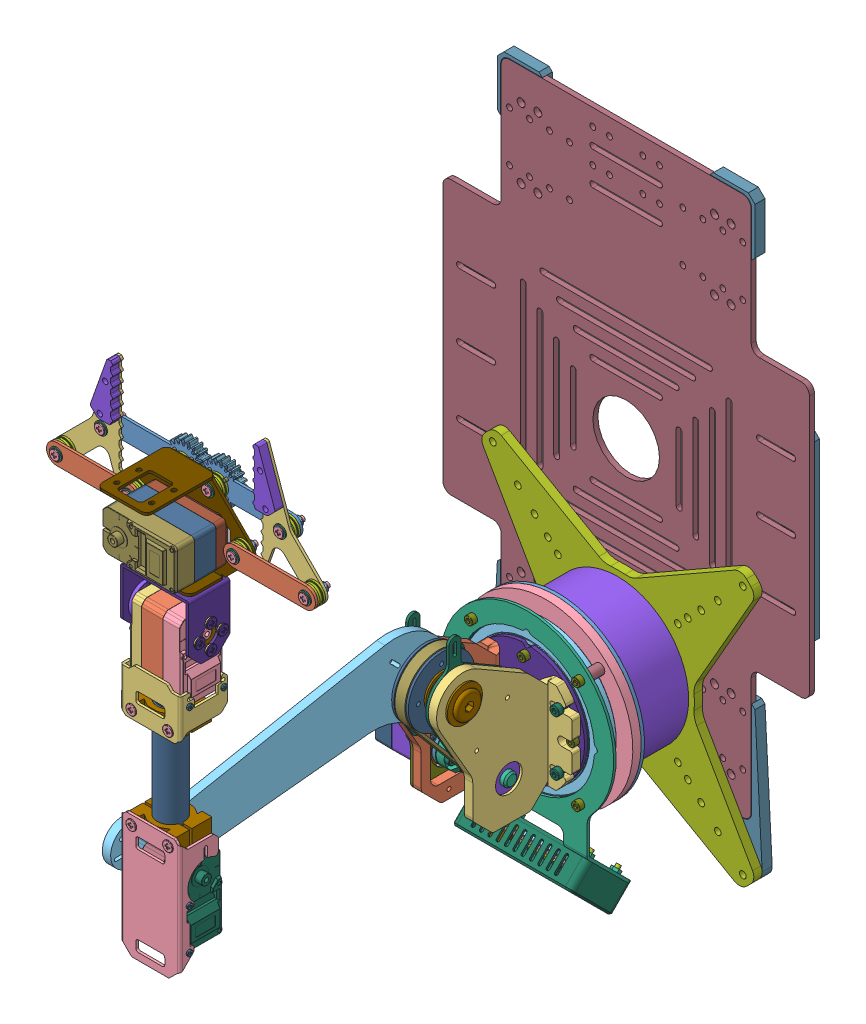
SolidWorks assembly RoArm-M1 STEP, configuration Default. Lengths in mm. (continued)
Components (placement in the parent): (continued)
- RoArm-M1 STEP(2)^RoArm-M1 STEP-1: RoArm-M1 STEP(2)^RoArm-M1 STEP [Default] at origin size (176.32 372.07 316.7) (virtual) (continued)
  - 银色金属螺丝 M2x8^RoArm-M1 STEP(2)_RoArm-M1 STEP-4: 银色金属螺丝 M2x8^RoArm-M1 STEP(2)_RoArm-M1 STEP [Default] at (19.3974 240.0016 262.6404) x (1 0 0) z (0 0 -1) size (3.6 3.6 9.22) (virtual)
  - 银色金属螺丝 M2x8^RoArm-M1 STEP(2)_RoArm-M1 STEP-5: 银色金属螺丝 M2x8^RoArm-M1 STEP(2)_RoArm-M1 STEP [Default] at (8.5797 240.0016 262.6404) x (1 0 0) z (0 0 -1) size (3.6 3.6 9.22) (virtual)
  - 银色金属螺丝 M2x8^RoArm-M1 STEP(2)_RoArm-M1 STEP-6: 银色金属螺丝 M2x8^RoArm-M1 STEP(2)_RoArm-M1 STEP [Default] at (-1.6026 229.8193 262.6404) x (1 0 0) z (0 0 -1) size (3.6 3.6 9.22) (virtual)
  - 银色金属螺丝 M2x8^RoArm-M1 STEP(2)_RoArm-M1 STEP-7: 银色金属螺丝 M2x8^RoArm-M1 STEP(2)_RoArm-M1 STEP [Default] at (8.5797 229.8193 262.6404) x (1 0 0) z (0 0 -1) size (3.6 3.6 9.22) (virtual)
  - 银色金属螺丝 M2x8^RoArm-M1 STEP(2)_RoArm-M1 STEP-8: 银色金属螺丝 M2x8^RoArm-M1 STEP(2)_RoArm-M1 STEP [Default] at (-1.6026 240.0016 262.6404) x (1 0 0) z (0 0 -1) size (3.6 3.6 9.22) (virtual)
  - 弹性垫片 M3^RoArm-M1 STEP(2)_RoArm-M1 STEP-24: 弹性垫片 M3^RoArm-M1 STEP(2)_RoArm-M1 STEP [Default] at (7 0 48.12) size (5.2 5.2 0.88) (virtual)
  - 弹性垫片 M3^RoArm-M1 STEP(2)_RoArm-M1 STEP-25: 弹性垫片 M3^RoArm-M1 STEP(2)_RoArm-M1 STEP [Default] at (0 -7 48.12) size (5.2 5.2 0.88) (virtual)
  - 弹性垫片 M3^RoArm-M1 STEP(2)_RoArm-M1 STEP-26: 弹性垫片 M3^RoArm-M1 STEP(2)_RoArm-M1 STEP [Default] at (-7 0 48.12) size (5.2 5.2 0.88) (virtual)
  - 弹性垫片 M3^RoArm-M1 STEP(2)_RoArm-M1 STEP-27: 弹性垫片 M3^RoArm-M1 STEP(2)_RoArm-M1 STEP [Default] at (0 7 48.12) size (5.2 5.2 0.88) (virtual)
  - 弹性垫片 M3^RoArm-M1 STEP(2)_RoArm-M1 STEP-28: 弹性垫片 M3^RoArm-M1 STEP(2)_RoArm-M1 STEP [Default] at (0 0 44.32) size (5.2 5.2 0.88) (virtual)
- vertical tool-1: vertical tool [Default] at (17.9615 -304.3961 -7.6382) x (0 1 0) z (1 0 0) size (68.1 225.29 14) (hidden)
- moebius_base_2-1: moebius_base_2 [Default] at (75.4807 148.9605 -3) x (0 1 0) z (0 0 1) size (324 220 3)
- bumper_roarm-1: bumper_roarm [Default] at (75.4807 148.9605 -3) x (0 -1 0) z (0 0 -1) size (357.68 220 6)
- display protector-1: display protector [Default] at (18.4653 807.4745 926.2172) x (0 -0.707107 -0.707107) z (0 -0.707107 0.707107) size (36.8 72 17.1)
Mates (geometry in assembly coordinates):
- InPlace1: in place: plane of RoArm-M1 STEP(2)^RoArm-M1 STEP-1/大扭矩云台模块^RoArm-M1 STEP(2)_RoArm-M1 STEP-1/云台从动侧^大扭矩云台模块_RoArm-M1 STEP(2)_RoArm-M1 STEP-1 through (17.9615 10.865 89.375) normal (1 0 0); plane of ? through (17.9615 0 0) normal (1 0 0); moOrthogonalPlaneRef_w of RoArm-M1 STEP(2)^RoArm-M1 STEP-1/大扭矩云台模块^RoArm-M1 STEP(2)_RoArm-M1 STEP-1/云台从动侧^大扭矩云台模块_RoArm-M1 STEP(2)_RoArm-M1 STEP-1 through (17.9615 10.865 89.375) normal (1 0 0); plane of ? through (17.9615 0 0) normal (0 1 0); plane of RoArm-M1 STEP(2)^RoArm-M1 STEP-1/大扭矩云台模块^RoArm-M1 STEP(2)_RoArm-M1 STEP-1/云台从动侧^大扭矩云台模块_RoArm-M1 STEP(2)_RoArm-M1 STEP-1 through (17.9615 10.865 89.375) normal (1 0 0); plane of ? through (17.9615 0 0) normal (0 0 -1); plane of RoArm-M1 STEP(2)^RoArm-M1 STEP-1/大扭矩云台模块^RoArm-M1 STEP(2)_RoArm-M1 STEP-1/云台从动侧^大扭矩云台模块_RoArm-M1 STEP(2)_RoArm-M1 STEP-1 through (17.9615 10.865 89.375) normal (1 0 0); unknown of vertical tool-1
- Coincident1: coincident aligned: plane of ?; plane of ?
- Coincident2: coincident aligned: moOrthogonalPlaneRef_w of RoArm-M1 STEP(2)^RoArm-M1 STEP-1/大扭矩云台模块^RoArm-M1 STEP(2)_RoArm-M1 STEP-1/云台从动侧^大扭矩云台模块_RoArm-M1 STEP(2)_RoArm-M1 STEP-1 through (17.9615 -304.3961 -7.6382) normal (0 0 1); plane of Part135^RoArm-M1 STEP-1 through (17.9615 -304.3961 -7.6382) normal (0 0 1)
- Coincident3: coincident anti-aligned: moOrthogonalPlaneRef_w of RoArm-M1 STEP(2)^RoArm-M1 STEP-1/大扭矩云台模块^RoArm-M1 STEP(2)_RoArm-M1 STEP-1/云台从动侧^大扭矩云台模块_RoArm-M1 STEP(2)_RoArm-M1 STEP-1 through (17.9615 -304.3961 -7.6382) normal (0 -1 0); plane of Part135^RoArm-M1 STEP-1 through (17.9615 -304.3961 -7.6382) normal (0 1 0)
- Coincident1: coincident anti-aligned: plane of RoArm-M1 STEP(2)^RoArm-M1 STEP-1/X型底座^RoArm-M1 STEP(2)_RoArm-M1 STEP-1 through (0 0 0) normal (0 0 -1); plane of moebius_base_2-1 through (-70 -45.25 0) normal (0 0 1)
- Concentric1: concentric anti-aligned: cylinder of RoArm-M1 STEP(2)^RoArm-M1 STEP-1/X型底座^RoArm-M1 STEP(2)_RoArm-M1 STEP-1 through (50 50 0) axis (0 0 1) radius 2; cylinder of moebius_base_2-1 through (50 50 0) axis (0 0 -1) radius 1.75
- Concentric2: concentric anti-aligned: cylinder of RoArm-M1 STEP(2)^RoArm-M1 STEP-1/X型底座^RoArm-M1 STEP(2)_RoArm-M1 STEP-1 through (-50 50 0) axis (0 0 1) radius 2; cylinder of moebius_base_2-1 through (-50 50 0) axis (0 0 -1) radius 1.75
- InPlace2: in place: plane of moebius_base_2-1 through (-70 -45.25 -3) normal (0 0 -1); plane of ? through (0 0 -3) normal (0 0 -1); plane of moebius_base_2-1 through (-70 -45.25 -3) normal (0 0 -1); plane of ? through (0 0 -3) normal (0 1 0); plane of moebius_base_2-1 through (-70 -45.25 -3) normal (0 0 -1); plane of ? through (0 0 -3) normal (-1 0 0); plane of moebius_base_2-1 through (-70 -45.25 -3) normal (0 0 -1); unknown of bumper_roarm-1
- Coincident2: coincident aligned: plane of ?; plane of ?
- Coincident3: coincident aligned: moOrthogonalPlaneRef_w of moebius_base_2-1 through (75.4807 148.9605 -3) normal (-1 0 0); plane of bumper_roarm-1 through (75.4807 148.9605 -3) normal (-1 0 0)
- Coincident4: coincident anti-aligned: moOrthogonalPlaneRef_w of moebius_base_2-1 through (75.4807 148.9605 -3) normal (0 1 0); plane of bumper_roarm-1 through (75.4807 148.9605 -3) normal (0 -1 0)
- InPlace3: in place: plane of RoArm-M1 STEP(2)^RoArm-M1 STEP-1/中心外侧PCB支架^RoArm-M1 STEP(2)_RoArm-M1 STEP-1 through (0 -33.6427 85.1) normal (0 -0.707107 0.707107); plane of ? through (0 -59.3713 59.3713) normal (0 -0.707107 0.707107); plane of RoArm-M1 STEP(2)^RoArm-M1 STEP-1/中心外侧PCB支架^RoArm-M1 STEP(2)_RoArm-M1 STEP-1 through (0 -33.6427 85.1) normal (0 -0.707107 0.707107); plane of ? through (0 -59.3713 59.3713) normal (0 0.707107 0.707107); plane of RoArm-M1 STEP(2)^RoArm-M1 STEP-1/中心外侧PCB支架^RoArm-M1 STEP(2)_RoArm-M1 STEP-1 through (0 -33.6427 85.1) normal (0 -0.707107 0.707107); plane of ? through (0 -59.3713 59.3713) normal (1 0 0); plane of RoArm-M1 STEP(2)^RoArm-M1 STEP-1/中心外侧PCB支架^RoArm-M1 STEP(2)_RoArm-M1 STEP-1 through (0 -33.6427 85.1) normal (0 -0.707107 0.707107); unknown of display protector-1
- Coincident5: coincident aligned: plane of ?; plane of ?
- Coincident6: coincident aligned: moOrthogonalPlaneRef_w of RoArm-M1 STEP(2)^RoArm-M1 STEP-1/中心外侧PCB支架^RoArm-M1 STEP(2)_RoArm-M1 STEP-1 through (18.4653 807.4745 926.2172) normal (1 0 0); plane of display protector-1 through (18.4653 807.4745 926.2172) normal (1 0 0)
- Coincident7: coincident anti-aligned: moOrthogonalPlaneRef_w of RoArm-M1 STEP(2)^RoArm-M1 STEP-1/中心外侧PCB支架^RoArm-M1 STEP(2)_RoArm-M1 STEP-1 through (18.4653 807.4745 926.2172) normal (0 0.707107 0.707107); plane of display protector-1 through (18.4653 807.4745 926.2172) normal (0 -0.707107 -0.707107)
